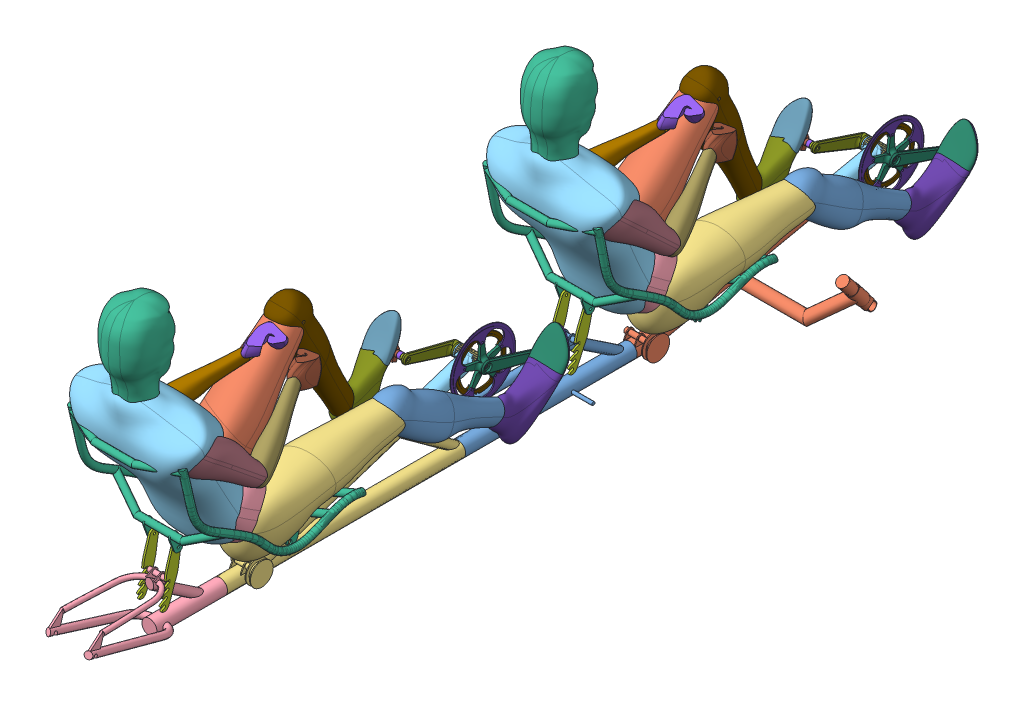
SolidWorks assembly Assembly, configuration Default. Lengths in mm.
Overall size (740 1661.62 3198).
94 component instances, 36 part files, 34 mates.
Components (placement in the parent):
- Part2_new-1: Part2_new [Default] at (126.0649 292.6359 159.5991) size (131.07 183.4 593.16)
- Part1-1: Part1 [Default] at (126.0649 424.1818 -521.9772) x (1 0 0) z (0 -0.207912 0.978148) size (740 154.63 706.7)
- Part3-1: Part3 [Default] at (126.0649 292.6359 743.5991) size (404.33 235.55 819.31)
- Part4-1: Part4 [Default] at (126.0649 292.6359 1554.5991) x (-1 0 0) z (0 0 -1) size (160.76 180.91 521.89)
- buis_voor_trappers-1: buis_voor_trappers [Default] at (126.0649 459.274 -687.0727) x (-1 0 0) z (0 0.207912 -0.978148) size (73.98 47.1 420)
- stoeltje2-2: stoeltje2 [Default] at (-57.7351 334.8998 1391.5439) x (0 0.625084 0.780558) z (-1 0 0) size (804.64 321.09 397.5)
- stoel_scharnierendstuk-1: stoel_scharnierendstuk [Default] at (166.2649 640.2114 1747.0277) x (0 -0.625619 -0.780129) z (-1 0 0) size (96.02 180.74 6.3)
- stoel_scharnierendstuk-2: stoel_scharnierendstuk [Default] at (89.5649 640.2114 1747.0277) x (0 -0.625619 -0.780129) z (-1 0 0) size (96.02 180.74 6.3)
- stoeltje2-3: stoeltje2 [Default] at (-58.6351 324.8364 -6.9963) x (0 0.647459 0.7621) z (-1 0 0) size (804.64 321.09 397.5)
- stoel_scharnierendstuk-3: stoel_scharnierendstuk [Default] at (88.6649 640.2908 332.8486) x (0 -0.690316 -0.723508) z (-1 0 0) size (96.02 180.74 6.3)
- stoel_scharnierendstuk-4: stoel_scharnierendstuk [Default] at (165.3649 640.2908 332.8486) x (0 -0.690316 -0.723508) z (-1 0 0) size (96.02 180.74 6.3)
- buis_voor_trappers-2: buis_voor_trappers [Default] at (126.0649 543.833 703.494) x (-1 0 0) z (0 0.309017 -0.951057) size (73.98 47.1 420)
- man and pedals-1: man and pedals [Default] at (-249.0769 -43.5363 1537.8604) x (0 0.160182 0.987087) z (-1 0 0) size (1682.46 1309.88 470.97)
  - man-1: man [Default] at (95.4934 600.9354 -375.0417) x (0 0 1) z (0.212729 0.977111 0) size (470.97 1501.17 1013.74)
    - l_hand-1: l_hand [Default] at (-75.061 -46.595 173.8025) x (0.830501 -0.201706 0.519214) z (0.434592 0.817704 -0.37748) size (75.14 87.95 126.56)
    - l_forearm-1: l_forearm [Default] at (-74.5383 -46.9587 172.8252) x (0.830501 -0.201706 0.519214) z (0.439679 0.80967 -0.388738) size (68.37 88.83 304.6)
    - l_uprarm-1: l_uprarm [Default] at (-25 -115.7538 113.8421) x (1 0 0) z (0 0.822399 0.568911) size (101.79 125.62 366.77)
    - r_hand-1: r_hand [Default] at (68.9738 -13.6688 334.1115) x (0.945068 0.323653 -0.045764) z (-0.296343 0.907441 0.297877) size (75.14 87.95 126.56)
    - r_forearm-1: r_forearm [Default] at (63.0967 -5.5024 270.4992) x (0.945068 0.323653 -0.045764) z (-0.300779 0.806246 -0.509411) size (68.37 88.83 304.6)
    - r_uprarm-1: r_uprarm [Default] at (25 -89.1244 75.7943) x (1 0 0) z (0 0.75752 0.652812) size (101.79 125.62 366.77)
    - Mirrorr_toe-1: Mirrorr_toe [Default] at (25 255.5166 312.7272) x (1 0 0) z (0 0.907972 0.419031) size (104.9 198.15 49.25)
    - r_toe-1: r_toe [Default] at (-25 -123.6394 355.9267) x (1 0 0) z (0 0.82548 0.564431) size (104.9 198.15 49.25)
    - Mirrorr_foot-1: Mirrorr_foot [Default] at (25 225.0717 389.8663) x (1 0 0) z (0 0.867996 0.496571) size (107.05 328.32 123.78)
    - r_foot_new-1: r_foot_new [Default] at (-25 -166.5093 426.9163) x (1 0 0) z (0 0.773145 0.634229) size (107.05 328.32 123.78)
    - Mirrorr_calf_new-1: Mirrorr_calf_new [Default] at (25 -129.5353 701.0398) x (-1 0 0) z (0 0.469055 0.883169) size (127.01 156.17 503.94)
    - r_calf_new-1: r_calf_new [Default] at (-25 -45.6447 258.7342) x (1 0 0) z (0 0.892742 0.450568) size (127.01 156.17 503.94)
    - Mirrorr_thigh-1: Mirrorr_thigh [Default] at (25 -4.1969 -33.3026) x (1 0 0) z (0 0.714896 -0.69923) size (222.9 246.68 623.17)
    - r_thigh-1: r_thigh [Default] at (-25 3.4243 -17.93) x (1 0 0) z (0 0.989334 -0.145662) size (222.9 246.68 623.17)
    - pelvis-1: pelvis [Default] x (1 0 0) z (0 0.866025 0.5) size (331.12 212.17 288.92)
    - torso-1: torso [Default] at (0 52.0745 -42.0543) x (1 0 0) z (0 0.422618 0.906308) size (470.97 355.44 644.94)
    - head-1: head [Default] at (0 263.8213 -97.7854) x (1 0 0) z (0 -0.004897 0.999988) size (179.98 221.25 518.74)
  - crank bb and pedals 68mm-1: crank bb and pedals 68mm [Default] at (-838.3364 589.4144 -403.2918) x (0 0 -1) z (0.910993 0.412423 0) size (287.85 236.51 405.65)
    - pedal_r_asm-1: pedal_r_asm [Default] at (23 118.6007 -6.7894) x (1 0 0) z (0 -0.086921 0.996215) size (92.68 78.48 31.62)
      - pedal_axle-1: pedal_axle [Default] at origin size (88.5 18 18)
      - pedal_nut-1: pedal_nut [Default] at (21.7178 0 0) x (1 0 0) z (0 -0.18399 0.982928) size (18 20 20)
      - pedal_body_r-1: pedal_body_r [Default] at (10.175 0 0) x (-1 0 0) z (0 -0.047279 -0.998882) size (62 77.24 28)
      - Angular Contact Ball Bearing_68_ISO-1: Angular Contact Ball Bearing_68_ISO [Default] at (85.0875 0 0) x (-1 0 0) z (0 -0.780525 -0.625124) size (3.18 12.7 12.7)
      - Angular Contact Ball Bearing_68_ISO-2: Angular Contact Ball Bearing_68_ISO [Default] at (22.0875 0 0) x (-1 0 0) z (0 -0.780525 -0.625124) size (3.18 12.7 12.7)
    - pedal_l_asm-1: pedal_l_asm [Default] at (-79.5001 18.292 307.5959) x (-1 0 0) z (0 -0.805203 -0.592999) size (92.68 57.51 81.9)
      - pedal_axle-1: pedal_axle [Default] at origin size (88.5 18 18)
      - pedal_nut-1: pedal_nut [Default] at (21.7178 0 0) x (1 0 0) z (0 -0.18399 0.982928) size (18 20 20)
      - pedal_body_l-1: pedal_body_l [Default] at (10.175 0 0) x (1 0 0) z (0 0.909932 0.414758) size (62 77.24 28)
      - Angular Contact Ball Bearing_68_ISO-1: Angular Contact Ball Bearing_68_ISO [Default] at (22.0875 0 0) size (3.18 12.7 12.7)
      - Angular Contact Ball Bearing_68_ISO-2: Angular Contact Ball Bearing_68_ISO [Default] at (85.0875 0 0) size (3.18 12.7 12.7)
    - bb-1: bb [Default] at (-28.2501 68.0984 150.2922) x (1 0 0) z (0 -0.981491 0.19151) size (108 49.07 49.07)
      - bb_shell-1: bb_shell [Default] at origin size (68 40 40)
      - bb_axle-1: bb_axle [Default] x (-1 0 0) z (0 -0.280049 -0.959986) size (108 19 19)
      - Angular Contact Ball Bearing_68_ISO_17X35X10_ISO 15 ABB - 1017 - 12,SI,NC,12_68-1: Angular Contact Ball Bearing_68_ISO_17X35X10_ISO 15 ABB - 1017 - 12,SI,NC,12_68 [Default] at (-29 0 0) x (-1 0 0) z (0 0.607904 0.794011) size (10 35 35)
      - Angular Contact Ball Bearing_68_ISO_17X35X10_ISO 15 ABB - 1017 - 12,SI,NC,12_68-2: Angular Contact Ball Bearing_68_ISO_17X35X10_ISO 15 ABB - 1017 - 12,SI,NC,12_68 [Default] at (29 0 0) x (1 0 0) z (0 0.448357 -0.893854) size (10 35 35)
    - crankarm_r-1: crankarm_r [Default] at (35 68.0984 150.2922) x (0 0.303966 -0.952683) z (-1 0 0) size (255 146.72 29)
    - crankarm_l-1: crankarm_l [Default] at (-91.5001 68.0984 150.2922) x (0 -0.303966 0.952683) z (1 0 0) size (200 40 25)
    - bigring_54-1: bigring_54 [Default] at (16 68.0984 150.2922) x (1 0 0) z (0 -0.005307 -0.999986) size (4 222.77 222.9)
    - smallring_42-1: smallring_42 [Default] at (8 68.0984 150.2922) x (1 0 0) z (0 -0.005307 -0.999986) size (4 174.23 174.39)
- man and pedals-2: man and pedals [Default] at (-249.0769 -66.8859 187.1846) x (0 0.230403 0.973095) z (-1 0 0) size (1682.46 1309.88 470.97)
  - man-1: man [Default] at (95.4934 600.9354 -375.0417) x (0 0 1) z (0.212729 0.977111 0) size (470.97 1501.17 1013.74)
    - l_hand-1: l_hand [Default] at (-75.061 -46.595 173.8025) x (0.830501 -0.201706 0.519214) z (0.434592 0.817704 -0.37748) size (75.14 87.95 126.56)
    - l_forearm-1: l_forearm [Default] at (-74.5383 -46.9587 172.8252) x (0.830501 -0.201706 0.519214) z (0.439679 0.80967 -0.388738) size (68.37 88.83 304.6)
    - l_uprarm-1: l_uprarm [Default] at (-25 -115.7538 113.8421) x (1 0 0) z (0 0.822399 0.568911) size (101.79 125.62 366.77)
    - r_hand-1: r_hand [Default] at (68.9738 -13.6688 334.1115) x (0.945068 0.323653 -0.045764) z (-0.296343 0.907441 0.297877) size (75.14 87.95 126.56)
    - r_forearm-1: r_forearm [Default] at (63.0967 -5.5024 270.4992) x (0.945068 0.323653 -0.045764) z (-0.300779 0.806246 -0.509411) size (68.37 88.83 304.6)
    - r_uprarm-1: r_uprarm [Default] at (25 -89.1244 75.7943) x (1 0 0) z (0 0.75752 0.652812) size (101.79 125.62 366.77)
    - Mirrorr_toe-1: Mirrorr_toe [Default] at (25 255.5166 312.7272) x (1 0 0) z (0 0.907972 0.419031) size (104.9 198.15 49.25)
    - r_toe-1: r_toe [Default] at (-25 -123.6394 355.9267) x (1 0 0) z (0 0.82548 0.564431) size (104.9 198.15 49.25)
    - Mirrorr_foot-1: Mirrorr_foot [Default] at (25 225.0717 389.8663) x (1 0 0) z (0 0.867996 0.496571) size (107.05 328.32 123.78)
    - r_foot_new-1: r_foot_new [Default] at (-25 -166.5093 426.9163) x (1 0 0) z (0 0.773145 0.634229) size (107.05 328.32 123.78)
    - Mirrorr_calf_new-1: Mirrorr_calf_new [Default] at (25 -129.5353 701.0398) x (-1 0 0) z (0 0.469055 0.883169) size (127.01 156.17 503.94)
    - r_calf_new-1: r_calf_new [Default] at (-25 -45.6447 258.7342) x (1 0 0) z (0 0.892742 0.450568) size (127.01 156.17 503.94)
    - Mirrorr_thigh-1: Mirrorr_thigh [Default] at (25 -4.1969 -33.3026) x (1 0 0) z (0 0.714896 -0.69923) size (222.9 246.68 623.17)
    - r_thigh-1: r_thigh [Default] at (-25 3.4243 -17.93) x (1 0 0) z (0 0.989334 -0.145662) size (222.9 246.68 623.17)
    - pelvis-1: pelvis [Default] x (1 0 0) z (0 0.866025 0.5) size (331.12 212.17 288.92)
    - torso-1: torso [Default] at (0 52.0745 -42.0543) x (1 0 0) z (0 0.422618 0.906308) size (470.97 355.44 644.94)
    - head-1: head [Default] at (0 263.8213 -97.7854) x (1 0 0) z (0 -0.004897 0.999988) size (179.98 221.25 518.74)
  - crank bb and pedals 68mm-1: crank bb and pedals 68mm [Default] at (-838.3364 589.4144 -403.2918) x (0 0 -1) z (0.910993 0.412423 0) size (287.85 236.51 405.65)
    - pedal_r_asm-1: pedal_r_asm [Default] at (23 118.6007 -6.7894) x (1 0 0) z (0 -0.086921 0.996215) size (92.68 78.48 31.62)
      - pedal_axle-1: pedal_axle [Default] at origin size (88.5 18 18)
      - pedal_nut-1: pedal_nut [Default] at (21.7178 0 0) x (1 0 0) z (0 -0.18399 0.982928) size (18 20 20)
      - pedal_body_r-1: pedal_body_r [Default] at (10.175 0 0) x (-1 0 0) z (0 -0.047279 -0.998882) size (62 77.24 28)
      - Angular Contact Ball Bearing_68_ISO-1: Angular Contact Ball Bearing_68_ISO [Default] at (85.0875 0 0) x (-1 0 0) z (0 -0.780525 -0.625124) size (3.18 12.7 12.7)
      - Angular Contact Ball Bearing_68_ISO-2: Angular Contact Ball Bearing_68_ISO [Default] at (22.0875 0 0) x (-1 0 0) z (0 -0.780525 -0.625124) size (3.18 12.7 12.7)
    - pedal_l_asm-1: pedal_l_asm [Default] at (-79.5001 18.292 307.5959) x (-1 0 0) z (0 -0.805203 -0.592999) size (92.68 57.51 81.9)
      - pedal_axle-1: pedal_axle [Default] at origin size (88.5 18 18)
      - pedal_nut-1: pedal_nut [Default] at (21.7178 0 0) x (1 0 0) z (0 -0.18399 0.982928) size (18 20 20)
      - pedal_body_l-1: pedal_body_l [Default] at (10.175 0 0) x (1 0 0) z (0 0.909932 0.414758) size (62 77.24 28)
      - Angular Contact Ball Bearing_68_ISO-1: Angular Contact Ball Bearing_68_ISO [Default] at (22.0875 0 0) size (3.18 12.7 12.7)
      - Angular Contact Ball Bearing_68_ISO-2: Angular Contact Ball Bearing_68_ISO [Default] at (85.0875 0 0) size (3.18 12.7 12.7)
    - bb-1: bb [Default] at (-28.2501 68.0984 150.2922) x (1 0 0) z (0 -0.981491 0.19151) size (108 49.07 49.07)
      - bb_shell-1: bb_shell [Default] at origin size (68 40 40)
      - bb_axle-1: bb_axle [Default] x (-1 0 0) z (0 -0.280049 -0.959986) size (108 19 19)
      - Angular Contact Ball Bearing_68_ISO_17X35X10_ISO 15 ABB - 1017 - 12,SI,NC,12_68-1: Angular Contact Ball Bearing_68_ISO_17X35X10_ISO 15 ABB - 1017 - 12,SI,NC,12_68 [Default] at (-29 0 0) x (-1 0 0) z (0 0.607904 0.794011) size (10 35 35)
      - Angular Contact Ball Bearing_68_ISO_17X35X10_ISO 15 ABB - 1017 - 12,SI,NC,12_68-2: Angular Contact Ball Bearing_68_ISO_17X35X10_ISO 15 ABB - 1017 - 12,SI,NC,12_68 [Default] at (29 0 0) x (1 0 0) z (0 0.448357 -0.893854) size (10 35 35)
    - crankarm_r-1: crankarm_r [Default] at (35 68.0984 150.2922) x (0 0.303966 -0.952683) z (-1 0 0) size (255 146.72 29)
    - crankarm_l-1: crankarm_l [Default] at (-91.5001 68.0984 150.2922) x (0 -0.303966 0.952683) z (1 0 0) size (200 40 25)
    - bigring_54-1: bigring_54 [Default] at (16 68.0984 150.2922) x (1 0 0) z (0 -0.005307 -0.999986) size (4 222.77 222.9)
    - smallring_42-1: smallring_42 [Default] at (8 68.0984 150.2922) x (1 0 0) z (0 -0.005307 -0.999986) size (4 174.23 174.39)
Mates (geometry in assembly coordinates):
- Coincident1: coincident anti-aligned: plane of Part2_new-1 through (126.0649 292.6359 159.5991) normal (0 0 -1); plane of Part1-1 through (126.0649 424.1818 159.5991) normal (0 0 1)
- Coincident2: coincident aligned: circle of Part2_new-1; circle of Part1-1
- Coincident3: coincident anti-aligned: plane of Part2_new-1 through (126.0649 292.6359 743.5991) normal (0 0 1); plane of Part3-1 through (126.0649 292.6359 743.5991) normal (0 0 -1)
- Coincident4: coincident aligned: circle of Part2_new-1; circle of Part3-1
- Coincident5: coincident anti-aligned: circle of Part3-1; circle of Part4-1
- Parallel1: parallel aligned: plane of Part4-1 through (141.6649 435.3478 1766.2105) normal (1 0 0); plane of assembly through (0 0 0) normal (1 0 0)
- Concentric1: concentric aligned: cylinder of Part1-1 through (126.0649 299.4348 64.9113) axis (0 0.207912 -0.978148) radius 24.2; cylinder of buis_voor_trappers-1 through (126.0649 376.1093 -295.8136) axis (0 0.207912 -0.978148) radius 23.55
- Parallel2: parallel aligned: plane of buis_voor_trappers-1 through (159.9649 459.274 -687.0727) normal (1 0 0); plane of assembly through (0 0 0) normal (1 0 0)
- Concentric2: concentric aligned: circle of stoeltje2-2; cylinder of stoel_scharnierendstuk-1 through (159.9649 523.9438 1741.0135) axis (1 0 0) radius 4
- Coincident6: coincident anti-aligned: plane of stoeltje2-2 through (166.2649 334.8998 1391.5439) normal (-1 0 0); plane of stoel_scharnierendstuk-1 through (166.2649 414.1289 1768.5814) normal (1 0 0)
- Concentric3: concentric aligned: cylinder of Part3-1 through (95.7649 370.5346 1346.5038) axis (1 0 0) radius 8.7; circle of stoeltje2-2
- Coincident9: coincident aligned: plane of Part3-1 through (87.7649 370.5346 1346.5038) normal (-1 0 0); plane of stoeltje2-2 through (87.7649 347.2826 1336.5427) normal (-1 0 0)
- Concentric4: concentric anti-aligned: circle of stoeltje2-2; circle of stoel_scharnierendstuk-2
- Coincident10: coincident anti-aligned: plane of stoeltje2-2 through (83.2649 334.8998 1391.5439) normal (1 0 0); plane of stoel_scharnierendstuk-2 through (83.2649 414.1289 1768.5814) normal (-1 0 0)
- Concentric5: concentric anti-aligned: circle of Part4-1; circle of stoel_scharnierendstuk-1
- Concentric6: concentric anti-aligned: circle of Part4-1; circle of stoel_scharnierendstuk-2
- Concentric7: concentric anti-aligned: circle of stoeltje2-3; circle of stoel_scharnierendstuk-4
- Coincident11: coincident anti-aligned: plane of stoeltje2-3 through (165.3649 324.8364 -6.9963) normal (-1 0 0); plane of stoel_scharnierendstuk-4 through (165.3649 416.8953 373.7421) normal (1 0 0)
- Concentric8: concentric anti-aligned: circle of stoeltje2-3; circle of stoel_scharnierendstuk-3
- Coincident12: coincident anti-aligned: plane of stoeltje2-3 through (82.3649 324.8364 -6.9963) normal (1 0 0); plane of stoel_scharnierendstuk-3 through (82.3649 416.8953 373.7421) normal (-1 0 0)
- Concentric9: concentric anti-aligned: cylinder of Part1-1 through (160.8649 359.1499 -53.051) axis (-1 0 0) radius 5; circle of stoeltje2-3
- Coincident13: coincident aligned: plane of Part1-1 through (160.8649 359.1499 -53.051) normal (1 0 0); plane of stoeltje2-3 through (160.8649 335.6188 -62.3335) normal (1 0 0)
- Concentric10: concentric aligned: cylinder of Part2_new-1 through (155.6149 437.8322 369.5574) axis (-1 0 0) radius 8.1; circle of stoel_scharnierendstuk-4
- Concentric11: concentric aligned: cylinder of Part2_new-1 through (155.6149 437.8322 369.5574) axis (-1 0 0) radius 8.1; circle of stoel_scharnierendstuk-3
- Concentric12: concentric aligned: cylinder of Part3-1 through (126.0649 267.2577 1554.705) axis (0 0.309017 -0.951057) radius 24.2; cylinder of buis_voor_trappers-2 through (126.0649 420.2262 1083.9166) axis (0 0.309017 -0.951057) radius 23.55
- Parallel3: parallel aligned: plane of Part3-1 through (194.8649 326.5203 1480.7991) normal (1 0 0); plane of buis_voor_trappers-2 through (159.9649 543.833 703.494) normal (1 0 0)
- Concentric13: concentric anti-aligned: cylinder of buis_voor_trappers-2 through (87.6649 543.833 703.494) axis (1 0 0) radius 17.15; cylinder of man and pedals-1/crank bb and pedals 68mm-1/bb-1/bb_shell-1 through (96.5823 543.833 703.494) axis (-1 0 0) radius 20
- Tangent3: tangent: cylinder of stoeltje2-2 through (52.7689 865.9102 1913.3238) axis (1 0 0) radius 11.25; face of man and pedals-1/man-1/torso-1
- Tangent4: tangent: cylinder of stoeltje2-2 through (52.7689 865.9102 1913.3238) axis (1 0 0) radius 11.25; face of man and pedals-1/man-1/torso-1
- Coincident15: coincident aligned: plane of buis_voor_trappers-2 through (159.9649 543.833 703.494) normal (1 0 0); plane of man and pedals-1/crank bb and pedals 68mm-1/bb-1/bb_shell-1 through (159.9649 556.2901 691.2029) normal (1 0 0)
- Lock1: lock: unknown of Part3-1; unknown of buis_voor_trappers-2
- Concentric14: concentric anti-aligned: cylinder of buis_voor_trappers-1 through (87.6649 459.274 -687.0727) axis (1 0 0) radius 17.15; cylinder of man and pedals-2/crank bb and pedals 68mm-1/bb-1/bb_shell-1 through (96.5823 459.274 -687.0727) axis (-1 0 0) radius 20
- Tangent5: tangent: cylinder of stoeltje2-3 through (51.8689 870.7564 499.1634) axis (1 0 0) radius 11.25; face of man and pedals-2/man-1/torso-1
- Coincident16: coincident aligned: plane of buis_voor_trappers-1 through (159.9649 459.274 -687.0727) normal (1 0 0); plane of man and pedals-2/crank bb and pedals 68mm-1/bb-1/bb_shell-1 through (159.9649 470.8197 -700.2236) normal (1 0 0)
